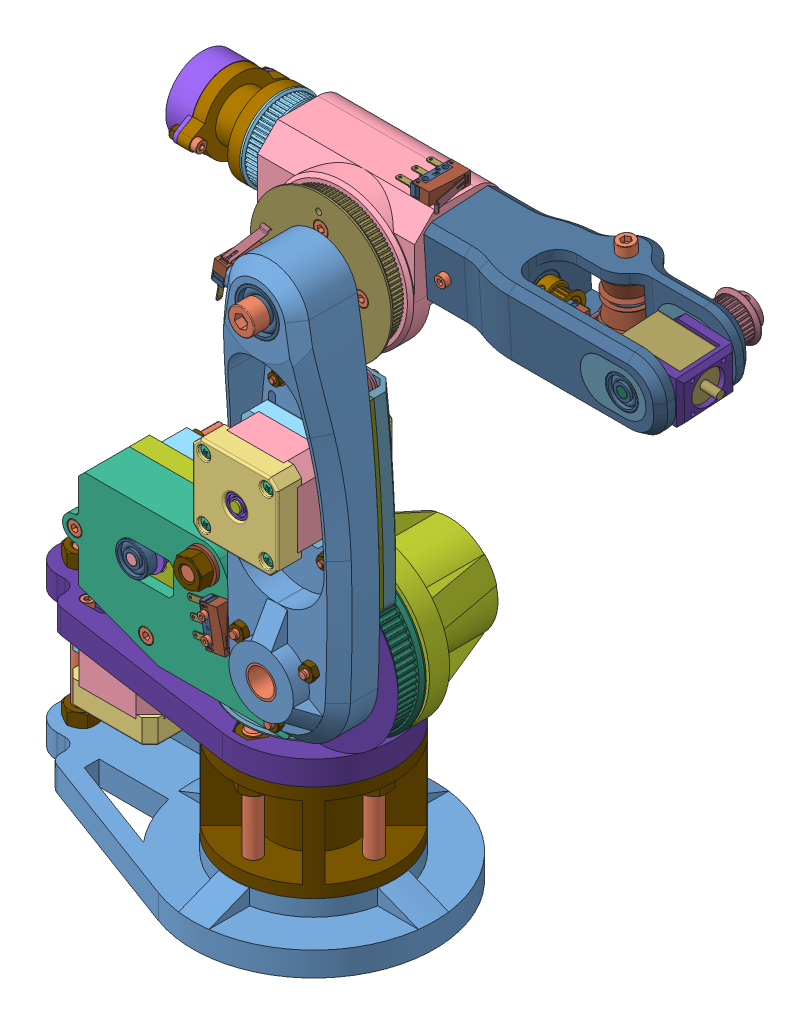
SolidWorks assembly Assem4_v2, configuration Default. Lengths in mm.
Overall size (329.84 338.53 142.9).
197 component instances, 53 part files, 399 mates.
Components (placement in the parent):
- Arm1v2-1: Arm1v2 [Default] at (144.3987 35.6213 88.0417) size (84.26 210 30)
- socket head cap screw_iso-2: socket head cap screw_iso [ISO 4762 M3 x 10 - 10N] at (128.8987 132.8213 85.0417) x (0 0 1) z (-1 0 0) size (13 5.5 5.5)
- socket head cap screw_iso-3: socket head cap screw_iso [ISO 4762 M3 x 10 - 10N] at (128.8987 101.8213 85.0417) x (0 0 1) z (-1 0 0) size (13 5.5 5.5)
- socket head cap screw_iso-4: socket head cap screw_iso [ISO 4762 M3 x 10 - 10N] at (159.8987 101.8213 85.0417) x (0 0 1) z (-1 0 0) size (13 5.5 5.5)
- socket head cap screw_iso-5: socket head cap screw_iso [ISO 4762 M3 x 10 - 10N] at (159.8987 132.8213 85.0417) x (0 0 1) z (-0.376004 -0.926618 0) size (13 5.5 5.5)
- NEMA 17 kiinalaiset-1: NEMA 17 kiinalaiset [Predeterminado] at (134.0032 112.7042 129.0417) x (-1 0 0) z (0 0 -1) size (42.3 42.3 56)
  - Base-1: Base [Predeterminado] at (-10.3955 4.6172 0) size (42.3 42.3 12)
  - Cuerpo-1: Cuerpo [Predeterminado] at (-10.3955 4.6172 10) size (42.3 42.3 16)
  - Tapa-1: Tapa [Predeterminado] at (-10.3955 4.6172 34) x (-1 0 0) z (0 0 -1) size (42.3 42.3 12)
  - pan cross head_am-1: pan cross head_am [B18.6.7M - M3 x 0.5 x 5 Type I Cross Recessed PHMS --5N] at (5.1045 20.1172 0.6) x (0 0 1) z (-0.896 0.444054 0) size (7.37 5.6 5.6)
  - pan cross head_am-2: pan cross head_am [B18.6.7M - M3 x 0.5 x 5 Type I Cross Recessed PHMS --5N] at (-25.8955 20.1172 0.6) x (0 0 1) z (-0.859432 0.51125 0) size (7.37 5.6 5.6)
  - pan cross head_am-3: pan cross head_am [B18.6.7M - M3 x 0.5 x 5 Type I Cross Recessed PHMS --5N] at (-25.8955 -10.8828 0.6) x (0 0 1) z (-0.91385 -0.406051 0) size (7.37 5.6 5.6)
  - pan cross head_am-4: pan cross head_am [B18.6.7M - M3 x 0.5 x 5 Type I Cross Recessed PHMS --5N] at (5.1045 -10.8828 0.6) x (0 0 1) z (-0.883632 0.468182 0) size (7.37 5.6 5.6)
  - Eje-1: Eje [Predeterminado] at (-10.3955 4.6172 0) x (0.574856 0.818255 0) z (0 0 1) size (5 5 56)
  - instrument ball bearing_68_am-2: instrument ball bearing_68_am [AFBMA 12.1.4.1 - 0050-11 - 10,SI,NC,10_68] at (-10.3955 4.6172 34) x (0 0 -1) z (0.925764 0.378103 0) size (3 11 11)
  - instrument ball bearing_68_am-4: instrument ball bearing_68_am [AFBMA 12.1.4.1 - 0050-11 - 10,SI,NC,10_68] at (-10.3955 4.6172 2.401) x (0 0 1) z (-0.993665 0.112385 0) size (3 11 11)
- GT2_16T_13x14-1: GT2_16T_13x14 [Конфигурация1] at (144.3987 117.3213 90.7117) x (0 0 -1) z (0.99998 0.006396 0) size (14.1 13 13)
- angular contact ball bearing_68_iso-1: angular contact ball bearing_68_iso [ISO 15 ABB - 108 - 8,SI,NC,8_68] at (144.3987 195.6213 91.5417) x (0 0 1) z (-0.999999 0.001328 0) size (7 22 22)
- angular contact ball bearing_68_iso-2: angular contact ball bearing_68_iso [ISO 15 ABB - 108 - 8,SI,NC,8_68] at (144.3987 195.6213 114.5417) x (0 0 -1) z (0.614558 -0.788871 0) size (7 22 22)
- socket head cap screw_iso-7: socket head cap screw_iso [ISO 4762 M8 x 80 - 28N] at (144.3987 195.6213 126.0417) x (0 0 -1) z (-0.988385 0.151973 0) size (88 13 13)
- plain washer normal grade a_iso-2: plain washer normal grade a_iso [Washer ISO 7089 - 8] at (144.3987 195.6213 88.0417) x (0 0 1) z (-0.999209 -0.03976 0) size (1.6 16 16)
- Pulley100Tv5-1: Pulley100Tv5 [Default] at (144.3987 195.6213 76.8417) x (0 0 1) z (0 1 0) size (15.6 70 70)
- socket head cap screw_iso-9: socket head cap screw_iso [ISO 4762 M3 x 25 - 18N] at (156.3987 150.6213 71.0417) x (0 0 1) z (-0.617239 0.786775 0) size (28 5.5 5.5)
- socket head cap screw_iso-10: socket head cap screw_iso [ISO 4762 M3 x 25 - 18N] at (132.3987 150.6213 71.0417) x (0 0 1) z (0.109591 0.993977 0) size (28 5.5 5.5)
- plain washer normal grade a_iso-4: plain washer normal grade a_iso [Washer ISO 7089 - 3] at (132.3987 150.6213 86.0417) x (0 0 1) z (-1 0 0) size (0.5 7 7)
- plain washer normal grade a_iso-5: plain washer normal grade a_iso [Washer ISO 7089 - 3] at (132.3987 150.6213 76.5417) x (0 0 1) z (-1 0 0) size (0.5 7 7)
- plain washer normal grade a_iso-6: plain washer normal grade a_iso [Washer ISO 7089 - 3] at (156.3987 150.6213 86.0417) x (0 0 1) z (-1 0 0) size (0.5 7 7)
- plain washer normal grade a_iso-7: plain washer normal grade a_iso [Washer ISO 7089 - 3] at (156.3987 150.6213 76.5417) x (0 0 1) z (-1 0 0) size (0.5 7 7)
- Toothless pulley 16t gt2-1: Toothless pulley 16t gt2 [Default] at (132.3987 150.6213 76.5417) x (0.593276 -0.804999 0) z (0 0 1) size (13 13 9)
- Toothless pulley 16t gt2-2: Toothless pulley 16t gt2 [Default] at (156.3987 150.6213 76.5417) x (0.93408 -0.357064 0) z (0 0 1) size (13 13 9)
- Arm 2.3-1: Arm 2.3 [Default] at (144.3987 35.6213 74.0417) x (0 0 1) z (-1 0 0) size (12 90.22 61.67)
- HTD3M 80T-1: HTD3M 80T [Default] at (144.3987 35.6213 86.4417) x (-0.5 -0.866025 0) z (0 0 -1) size (80 80 12.4)
- Arm 4.3-1: Arm 4.3 [Default] at (144.3987 35.6213 88.0417) x (0 0 -1) z (1 0 0) size (12 90.22 61.67)
- HTD80T 2mm spacer-1: HTD80T 2mm spacer [Default] at (144.3987 35.6213 88.0417) x (0.5 -0.866025 0) z (0.866025 0.5 0) size (80 1.6 80)
- socket head cap screw_iso-11: socket head cap screw_iso [ISO 4762 M3 x 25 - 18N] at (156.3987 83.6213 71.0417) x (0 0 1) z (-0.617239 0.786775 0) size (28 5.5 5.5)
- socket head cap screw_iso-12: socket head cap screw_iso [ISO 4762 M3 x 25 - 18N] at (132.3987 83.6213 71.0417) x (0 0 1) z (-0.617239 0.786775 0) size (28 5.5 5.5)
- socket head cap screw_iso-14: socket head cap screw_iso [ISO 4762 M4 x 35 - 20N] at (161.7192 45.6213 74.0417) x (0 0 1) z (-1 0 0) size (39 7 7)
- socket head cap screw_iso-15: socket head cap screw_iso [ISO 4762 M4 x 35 - 20N] at (127.0782 45.6213 74.0417) x (0 0 1) z (-1 0 0) size (39 7 7)
- socket head cap screw_iso-16: socket head cap screw_iso [ISO 4762 M4 x 35 - 20N] at (144.3987 15.6213 74.0417) x (0 0 1) z (-1 0 0) size (39 7 7)
- hex nut style 1 gradeab_iso-2: hex nut style 1 gradeab_iso [ISO - 4032 - M4 - W - N] at (161.7192 45.6213 108.0417) x (-0.89075 -0.454494 0) z (0 0 -1) size (7 8.08 3.2)
- hex nut style 1 gradeab_iso-3: hex nut style 1 gradeab_iso [ISO - 4032 - M4 - W - N] at (144.3987 15.6213 108.0417) x (-0.861185 -0.508291 0) z (0 0 -1) size (7 8.08 3.2)
- hex nut style 1 gradeab_iso-4: hex nut style 1 gradeab_iso [ISO - 4032 - M4 - W - N] at (127.0782 45.6213 108.0417) x (-0.923728 -0.383049 0) z (0 0 -1) size (7 8.08 3.2)
- plain washer normal grade a_iso-12: plain washer normal grade a_iso [Washer ISO 7089 - 3] at (132.3987 150.6213 95.0417) x (0 0 -1) z (1 0 0) size (0.5 7 7)
- plain washer normal grade a_iso-13: plain washer normal grade a_iso [Washer ISO 7089 - 3] at (156.3987 150.6213 95.0417) x (0 0 -1) z (1 0 0) size (0.5 7 7)
- plain washer normal grade a_iso-14: plain washer normal grade a_iso [Washer ISO 7089 - 3] at (132.3987 83.6213 95.0417) x (0 0 -1) z (1 0 0) size (0.5 7 7)
- plain washer normal grade a_iso-15: plain washer normal grade a_iso [Washer ISO 7089 - 3] at (156.3987 83.6213 95.0417) x (0 0 -1) z (1 0 0) size (0.5 7 7)
- hex nut style 1 gradeab_iso-6: hex nut style 1 gradeab_iso [ISO - 4032 - M3 - W - N] at (156.3987 150.6213 95.5417) x (-0.938673 -0.34481 0) z (0 0 -1) size (5.5 6.35 2.4)
- hex nut style 1 gradeab_iso-7: hex nut style 1 gradeab_iso [ISO - 4032 - M3 - W - N] at (132.3987 150.6213 95.5417) x (-0.945652 -0.32518 0) z (0 0 -1) size (5.5 6.35 2.4)
- hex nut style 1 gradeab_iso-8: hex nut style 1 gradeab_iso [ISO - 4032 - M3 - W - N] at (132.3987 83.6213 95.5417) x (-0.632186 -0.774817 0) z (0 0 -1) size (5.5 6.35 2.4)
- hex nut style 1 gradeab_iso-11: hex nut style 1 gradeab_iso [ISO - 4032 - M3 - W - N] at (156.3987 83.6213 95.5417) x (-0.632186 -0.774817 0) z (0 0 -1) size (5.5 6.35 2.4)
- angular contact ball bearing_68_iso-3: angular contact ball bearing_68_iso [ISO 15 ABB - 1015 - 12,SI,NC,12_68] at (174.8987 210.6213 52.4417) x (1 0 0) z (0 -0.976606 0.215038) size (9 32 32)
- angular contact ball bearing_68_iso-4: angular contact ball bearing_68_iso [ISO 15 ABB - 1015 - 12,SI,NC,12_68] at (105.8987 210.6213 52.4417) x (1 0 0) z (0 -0.4108 -0.911725) size (9 32 32)
- 100mm aluputki-1: 100mm aluputki [Default] at (66.1987 210.6213 52.4417) x (1 0 0) z (0 0.412587 -0.910918) size (145 15 15)
- 90mm aluputki-1: 90mm aluputki [Default] at (144.3987 35.6213 26.0417) x (-0.632641 -0.774445 0) z (0 0 1) size (15 15 90)
- angular contact ball bearing_68_iso-5: angular contact ball bearing_68_iso [ISO 15 ABB - 1015 - 12,SI,NC,12_68] at (144.3987 35.6213 67.9417) x (0 0 1) z (-0.817534 0.575881 0) size (9 32 32)
- angular contact ball bearing_68_iso-6: angular contact ball bearing_68_iso [ISO 15 ABB - 1015 - 12,SI,NC,12_68] at (144.3987 35.6213 26.9417) x (0 0 1) z (-0.997702 0.067753 0) size (9 32 32)
- 15mm 1.6 rikka-1: 15mm 1.6 rikka [Default] at (144.3987 35.6213 74.0417) x (0 0 -1) z (1 -0.000633 0) size (1.6 22 22)
- socket head cap screw_iso-23: socket head cap screw_iso [ISO 4762 M8 x 40 - 28N] at (94.3987 50.6213 54.4417) x (0 0 1) z (-0.999928 0.012039 0) size (48 13 13)
- angular contact ball bearing_68_iso-7: angular contact ball bearing_68_iso [ISO 15 ABB - 108 - 8,SI,NC,8_68] at (94.3987 50.6213 77.5417) x (0 0 -1) z (0.936997 0.349338 0) size (7 22 22)
- Arm2Mountv2-1: Arm2Mountv2 [Default] at (144.3987 195.6213 76.8417) x (0 0 -1) z (1 0 0) size (46 80 78)
- Pulley60Tv2-1: Pulley60Tv2 [Default] at (100.1987 210.6213 52.4417) x (0 0.659878 0.751372) z (-1 0 0) size (40 40 10)
- GT2_16T_13x14-2: GT2_16T_13x14 [Конфигурация1] at (104.8687 168.7922 48.8417) x (-1 0 0) z (0 -0.490303 -0.871552) size (14.1 13 13)
- 15mm rikka 1.2mm-1: 15mm rikka 1.2mm [Default] at (101.3987 210.6213 52.4417) x (0 -0.416782 0.909006) z (-1 0 0) size (20 20 1.2)
- Nema 14 stepper-1: Nema 14 stepper [Default] at (129.3987 168.7922 48.8417) x (0 0 1) z (-1 0 0) size (35.2 35.2 32.5)
- Nema 14 Round stepper-2: Nema 14 Round stepper [Default] at (51.6987 210.6213 52.4417) x (0 0.064696 -0.997905) z (1 0 0) size (50.5 36.5 20)
- Motor 5 adapter-1: Motor 5 adapter [Default] at (90.1987 210.6213 52.4417) x (-1 0 0) z (0 0.064696 -0.997905) size (26 40 50.5)
- socket head cap screw_iso-33: socket head cap screw_iso [ISO 4762 M3 x 12 - 12N] at (73.1987 209.2012 74.3457) x (-1 0 0) z (0 -0.223084 0.974799) size (15 5.5 5.5)
- socket head cap screw_iso-34: socket head cap screw_iso [ISO 4762 M3 x 12 - 12N] at (73.1987 212.0414 30.5377) x (-1 0 0) z (0 -0.996697 0.081212) size (15 5.5 5.5)
- hex nut style 1 gradeab_iso-15: hex nut style 1 gradeab_iso [ISO - 4032 - M3 - W - N] at (62.1987 212.0414 30.5377) x (0 -0.893584 -0.448895) z (1 0 0) size (5.5 6.35 2.4)
- hex nut style 1 gradeab_iso-16: hex nut style 1 gradeab_iso [ISO - 4032 - M3 - W - N] at (62.1987 209.2012 74.3457) x (0 -0.971525 -0.236939) z (1 0 0) size (5.5 6.35 2.4)
- plain washer normal grade a_iso-17: plain washer normal grade a_iso [Washer ISO 7089 - 8] at (94.3987 50.6213 72.4417) x (0 0 -1) z (1 0 0) size (1.6 16 16)
- plain washer normal grade a_iso-18: plain washer normal grade a_iso [Washer ISO 7089 - 8] at (94.3987 50.6213 89.6417) x (0 0 1) z (-1 0 0) size (1.6 16 16)
- angular contact ball bearing_68_iso-8: angular contact ball bearing_68_iso [ISO 15 ABB - 108 - 8,SI,NC,8_68] at (94.3987 50.6213 84.5417) x (0 0 -1) z (0.994052 0.108909 0) size (7 22 22)
- plain washer normal grade a_iso-20: plain washer normal grade a_iso [Washer ISO 7089 - 8] at (94.3987 50.6213 94.6417) x (0 0 -1) z (0.534163 0.845382 0) size (1.6 16 16)
- hex nut style 1 gradeab_iso-18: hex nut style 1 gradeab_iso [ISO - 4032 - M8 - W - N] at (94.3987 50.6213 96.2417) x (-0.975025 0.222094 0) z (0 0 -1) size (13 15.01 6.8)
- Microswitch-SS-3GL13SL-1: Microswitch-SS-3GL13SL [Default] at (90.1948 35.3075 79.4243) x (0.173648 -0.984808 0) z (0 0 1) size (23.17 24.53 6.3)
  - limit-switch-bottomcase-1: limit-switch-bottomcase [Default] at (4.8379 12.1903 15.2174) size (19.75 5.4 6.2)
  - limit-switch-top-case-1: limit-switch-top-case [Default] at (4.8379 12.1903 15.2174) size (19.75 9.81 6.3)
  - pins-1: pins [Default] at (4.7048 12.1903 18.0824) size (18.65 8.8 0.47)
  - switch_lever-1: switch_lever [Default] at (4.2786 20.8228 20.3174) x (0 0 -1) z (0.981158 -0.193205 0) size (4 3.58 20.93)
- socket head cap screw_iso-36: socket head cap screw_iso [ISO 4762 M2 x 10 - 10N] at (101.319 35.6213 102.8417) x (0 0 -1) z (1 0 0) size (12 3.8 3.8)
- socket head cap screw_iso-37: socket head cap screw_iso [ISO 4762 M2 x 10 - 10N] at (103.0555 25.7732 102.8417) x (0 0 -1) z (1 0 0) size (12 3.8 3.8)
- socket head cap screw_iso-39: socket head cap screw_iso [ISO 4762 M3 x 8 - 8N] at (101.3987 181.7922 35.8417) x (1 0 0) z (0 -0.369885 0.929078) size (11 5.5 5.5)
- socket head cap screw_iso-40: socket head cap screw_iso [ISO 4762 M3 x 8 - 8N] at (101.3987 181.7922 61.8417) x (1 0 0) z (0 -0.369885 0.929078) size (11 5.5 5.5)
- socket head cap screw_iso-41: socket head cap screw_iso [ISO 4762 M3 x 8 - 8N] at (101.3987 155.7922 61.8417) x (1 0 0) z (0 -0.369885 0.929078) size (11 5.5 5.5)
- socket head cap screw_iso-42: socket head cap screw_iso [ISO 4762 M3 x 8 - 8N] at (101.3987 155.7922 35.8417) x (1 0 0) z (0 0.072717 0.997353) size (11 5.5 5.5)
- socket head cap screw_iso-44: socket head cap screw_iso [ISO 4762 M4 x 16 - 16N] at (144.3987 215.6213 86.4417) x (0 0 -1) z (1 0 0) size (20 7 7)
- socket head cap screw_iso-46: socket head cap screw_iso [ISO 4762 M4 x 16 - 16N] at (164.3987 195.6213 86.4417) x (0 0 -1) z (1 0 0) size (20 7 7)
- socket head cap screw_iso-47: socket head cap screw_iso [ISO 4762 M4 x 16 - 16N] at (144.3987 175.6213 86.4417) x (0 0 -1) z (1 0 0) size (20 7 7)
- socket head cap screw_iso-48: socket head cap screw_iso [ISO 4762 M4 x 16 - 16N] at (124.3987 195.6213 86.4417) x (0 0 -1) z (0.806628 0.591059 0) size (20 7 7)
- hex nut style 1 gradeab_iso-19: hex nut style 1 gradeab_iso [ISO - 4032 - M8 - W - N] at (144.3987 195.6213 45.8417) x (0.866025 -0.5 0) z (0 0 1) size (13 15.01 6.8)
- Microswitch-SS-3GL13SL-2: Microswitch-SS-3GL13SL [Default] at (133.5542 178.7224 93.9191) x (0 0 1) z (-0.985156 0.171661 0) size (23.17 24.53 6.3)
  - limit-switch-bottomcase-1: limit-switch-bottomcase [Default] at (4.8379 12.1903 15.2174) size (19.75 5.4 6.2)
  - limit-switch-top-case-1: limit-switch-top-case [Default] at (4.8379 12.1903 15.2174) size (19.75 9.81 6.3)
  - pins-1: pins [Default] at (4.7048 12.1903 18.0824) size (18.65 8.8 0.47)
  - switch_lever-1: switch_lever [Default] at (4.2786 20.8228 20.3174) x (0 0 -1) z (0.981158 -0.193205 0) size (4 3.58 20.93)
- Pulley100TBase-2: Pulley100TBase [Default] at (106.8987 -6.3787 52.4417) x (0 -1 0) z (1 0 0) size (9.3 70 70)
- socket head cap screw_iso-50: socket head cap screw_iso [ISO 4762 M4 x 35 - 20N] at (65.8987 5.6213 94.6417) x (0 0 -1) z (0.847074 -0.531475 0) size (39 7 7)
- hex nut style 1 gradeab_iso-21: hex nut style 1 gradeab_iso [ISO - 4032 - M4 - W - N] at (65.8987 5.6213 62.4417) x (-0.520571 -0.853818 0) z (0 0 1) size (7 8.08 3.2)
- socket head cap screw_iso-54: socket head cap screw_iso [ISO 4762 M4 x 30 - 20N] at (30.3987 34.1213 94.6417) x (0 0 -1) z (0.979653 0.200699 0) size (34 7 7)
- hex nut style 1 gradeab_iso-22: hex nut style 1 gradeab_iso [ISO - 4032 - M4 - W - N] at (30.3987 34.1213 67.4417) x (0.5 -0.866025 0) z (0 0 1) size (7 8.08 3.2)
- hex nut style 1 gradeab_iso-23: hex nut style 1 gradeab_iso [ISO - 4032 - M8 - W - N] at (106.8987 42.6213 52.4417) x (0.866025 0 -0.5) z (0 -1 0) size (13 15.01 6.8)
- thrust ball bearing_68_iso-1: thrust ball bearing_68_iso [ISO 104 - 112035 - B,14,SI,NC,14_68] at (106.8987 -17.6787 52.4417) x (0 -1 0) z (-0.999778 0 -0.021086) size (10 35 35)
- thrust ball bearing_68_iso-2: thrust ball bearing_68_iso [ISO 104 - 112035 - B,14,SI,NC,14_68] at (106.8987 -81.6787 52.4417) x (0 1 0) z (0.068397 0 0.997658) size (10 35 35)
- Bottom spacer-1: Bottom spacer [Default] at (106.8987 -4.3787 52.4417) x (0.893445 0 -0.449173) z (-0.449173 0 -0.893445) size (70 2 70)
- Baseplate-1: Baseplate [Default] at (106.8987 -31.6787 52.4417) x (-1 0 0) z (0 0 -1) size (167.5 12 80)
- Bottom Tube-1: Bottom Tube [Default] at (106.8987 -31.6787 52.4417) x (0 0 -1) z (-1 0 0) size (80 48 80)
- angular contact ball bearing_68_iso-9: angular contact ball bearing_68_iso [ISO 15 ABB - 1015 - 12,SI,NC,12_68] at (106.8987 -27.1787 52.4417) x (0 -1 0) z (0 0 1) size (9 32 32)
- angular contact ball bearing_68_iso-10: angular contact ball bearing_68_iso [ISO 15 ABB - 1015 - 12,SI,NC,12_68] at (106.8987 -72.1787 52.4417) x (0 -1 0) z (0.009581 0 0.999954) size (9 32 32)
- Bottom support-1: Bottom support [Default] at (106.8987 -87.6787 52.4417) x (-1 0 0) z (0 0 -1) size (187.5 20 120)
- socket head cap screw_iso-58: socket head cap screw_iso [ISO 4762 M4 x 20 - 20N] at (131.8987 -15.6787 52.4417) x (0 1 0) z (0 0 1) size (24 7 7)
- hex nut style 1 gradeab_iso-24: hex nut style 1 gradeab_iso [ISO - 4032 - M4 - W - N] at (131.8987 5.6213 52.4417) x (-0.994978 0 0.100092) z (0 -1 0) size (7 8.08 3.2)
- NEMA 17 kiinalaiset-2: NEMA 17 kiinalaiset [Predeterminado] at (15.2032 -63.6787 47.8246) x (-1 0 0) z (0 1 0) size (42.3 42.3 56)
  - Base-1: Base [Predeterminado] at (-10.3955 4.6172 0) size (42.3 42.3 12)
  - Cuerpo-1: Cuerpo [Predeterminado] at (-10.3955 4.6172 10) size (42.3 42.3 16)
  - Tapa-1: Tapa [Predeterminado] at (-10.3955 4.6172 34) x (-1 0 0) z (0 0 -1) size (42.3 42.3 12)
  - pan cross head_am-1: pan cross head_am [B18.6.7M - M3 x 0.5 x 5 Type I Cross Recessed PHMS --5N] at (5.1045 20.1172 0.6) x (0 0 1) z (-0.896 0.444054 0) size (7.37 5.6 5.6)
  - pan cross head_am-2: pan cross head_am [B18.6.7M - M3 x 0.5 x 5 Type I Cross Recessed PHMS --5N] at (-25.8955 20.1172 0.6) x (0 0 1) z (-0.859432 0.51125 0) size (7.37 5.6 5.6)
  - pan cross head_am-3: pan cross head_am [B18.6.7M - M3 x 0.5 x 5 Type I Cross Recessed PHMS --5N] at (-25.8955 -10.8828 0.6) x (0 0 1) z (-0.91385 -0.406051 0) size (7.37 5.6 5.6)
  - pan cross head_am-4: pan cross head_am [B18.6.7M - M3 x 0.5 x 5 Type I Cross Recessed PHMS --5N] at (5.1045 -10.8828 0.6) x (0 0 1) z (-0.883632 0.468182 0) size (7.37 5.6 5.6)
  - Eje-1: Eje [Predeterminado] at (-10.3955 4.6172 0) x (0.574856 0.818255 0) z (0 0 1) size (5 5 56)
  - instrument ball bearing_68_am-2: instrument ball bearing_68_am [AFBMA 12.1.4.1 - 0050-11 - 10,SI,NC,10_68] at (-10.3955 4.6172 34) x (0 0 -1) z (0.925764 0.378103 0) size (3 11 11)
  - instrument ball bearing_68_am-4: instrument ball bearing_68_am [AFBMA 12.1.4.1 - 0050-11 - 10,SI,NC,10_68] at (-10.3955 4.6172 2.401) x (0 0 1) z (-0.993665 0.112385 0) size (3 11 11)
- socket head cap screw_iso-60: socket head cap screw_iso [ISO 4762 M3 x 10 - 10N] at (10.0987 -19.6787 36.9417) x (0 -1 0) z (0.275126 0 0.961408) size (13 5.5 5.5)
- socket head cap screw_iso-61: socket head cap screw_iso [ISO 4762 M3 x 10 - 10N] at (10.0987 -19.6787 67.9417) x (0 -1 0) z (0 0 1) size (13 5.5 5.5)
- socket head cap screw_iso-62: socket head cap screw_iso [ISO 4762 M3 x 10 - 10N] at (41.0987 -19.6787 36.9417) x (0 -1 0) z (0 0 1) size (13 5.5 5.5)
- socket head cap screw_iso-63: socket head cap screw_iso [ISO 4762 M3 x 10 - 10N] at (41.0987 -19.6787 67.9417) x (0 -1 0) z (0 0 1) size (13 5.5 5.5)
- GT2_16T_13x14-3: GT2_16T_13x14 [Конфигурация1] at (25.5987 -20.2487 52.4417) x (0 1 0) z (0 0 1) size (14.1 13 13)
- socket head cap screw_iso-65: socket head cap screw_iso [ISO 4762 M8 x 70 - 28N] at (106.8987 -97.6787 22.4417) x (0 1 0) z (0 0 1) size (78 13 13)
- socket head cap screw_iso-66: socket head cap screw_iso [ISO 4762 M8 x 70 - 28N] at (76.8987 -97.6787 52.4417) x (0 1 0) z (0 0 1) size (78 13 13)
- socket head cap screw_iso-67: socket head cap screw_iso [ISO 4762 M8 x 70 - 28N] at (106.8987 -97.6787 82.4417) x (0 1 0) z (0 0 1) size (78 13 13)
- socket head cap screw_iso-68: socket head cap screw_iso [ISO 4762 M8 x 70 - 28N] at (136.8987 -97.6787 52.4417) x (0 1 0) z (0 0 1) size (78 13 13)
- hex nut style 1 gradeab_iso-26: hex nut style 1 gradeab_iso [ISO - 4032 - M8 - D - N] at (106.8987 -44.4787 22.4417) x (1 0 0) z (0 -1 0) size (13 15.01 6.8)
- hex nut style 1 gradeab_iso-27: hex nut style 1 gradeab_iso [ISO - 4032 - M8 - D - N] at (136.8987 -44.4787 52.4417) x (1 0 0) z (0 -1 0) size (13 15.01 6.8)
- hex nut style 1 gradeab_iso-28: hex nut style 1 gradeab_iso [ISO - 4032 - M8 - D - N] at (106.8987 -44.4787 82.4417) x (1 0 0) z (0 -1 0) size (13 15.01 6.8)
- hex nut style 1 gradeab_iso-29: hex nut style 1 gradeab_iso [ISO - 4032 - M8 - D - N] at (76.8987 -43.4787 52.4417) x (1 0 0) z (0 -1 0) size (13 15.01 6.8)
- hex nut style 1 gradeab_iso-30: hex nut style 1 gradeab_iso [ISO - 4032 - M8 - D - N] at (106.8987 -20.8787 82.4417) x (0.866025 0 -0.5) z (0 1 0) size (13 15.01 6.8)
- hex nut style 1 gradeab_iso-31: hex nut style 1 gradeab_iso [ISO - 4032 - M8 - D - N] at (136.8987 -27.6787 52.4417) x (1 0 0) z (0 -1 0) size (13 15.01 6.8)
- hex nut style 1 gradeab_iso-32: hex nut style 1 gradeab_iso [ISO - 4032 - M8 - D - N] at (106.8987 -20.8787 22.4417) x (-0.866025 0 0.5) z (0 1 0) size (13 15.01 6.8)
- hex nut style 1 gradeab_iso-33: hex nut style 1 gradeab_iso [ISO - 4032 - M8 - D - N] at (76.8987 -27.6787 52.4417) x (1 0 0) z (0 -1 0) size (13 15.01 6.8)
- hex bolt gradeab_iso-2: hex bolt gradeab_iso [ISO 4014 - M8 x 80 x 80-N] at (-8.1013 -98.9787 52.4417) x (0 1 0) z (0 0 1) size (85.3 15.01 13)
- hex nut style 1 gradeab_iso-35: hex nut style 1 gradeab_iso [ISO - 4032 - M8 - D - N] at (-8.1013 -87.6787 52.4417) x (1 0 0) z (0 -1 0) size (13 15.01 6.8)
- hex nut style 1 gradeab_iso-36: hex nut style 1 gradeab_iso [ISO - 4032 - M8 - D - N] at (-8.1013 -38.4787 52.4417) x (1 0 0) z (0 -1 0) size (13 15.01 6.8)
- hex nut style 1 gradeab_iso-37: hex nut style 1 gradeab_iso [ISO - 4032 - M8 - D - N] at (-8.1013 -19.6787 52.4417) x (1 0 0) z (0 -1 0) size (13 15.01 6.8)
- Nema 17 planetary 5 to 1 gearbox-1: Nema 17 planetary 5 to 1 gearbox [Default] at (59.3987 35.6213 -13.8583) size (42.3 42.3 79.3)
- HTD pulley adapter-1: HTD pulley adapter [Default] at (59.3987 35.6213 54.4417) x (0.999676 0.02547 0) z (0 0 1) size (12 12 41)
- Motor1 spacer-1: Motor1 spacer [Default] at (59.3987 35.6213 47.4417) size (45 45 15)
- socket head cap screw_iso-70: socket head cap screw_iso [ISO 4762 M3 x 10 - 10N] at (49.4992 45.5208 57.4417) x (0 0 -1) z (1 0 0) size (13 5.5 5.5)
- socket head cap screw_iso-71: socket head cap screw_iso [ISO 4762 M3 x 10 - 10N] at (69.2982 45.5208 57.4417) x (0 0 -1) z (1 0 0) size (13 5.5 5.5)
- socket head cap screw_iso-72: socket head cap screw_iso [ISO 4762 M3 x 10 - 10N] at (69.2982 25.7218 57.4417) x (0 0 -1) z (1 0 0) size (13 5.5 5.5)
- socket head cap screw_iso-73: socket head cap screw_iso [ISO 4762 M3 x 10 - 10N] at (49.4992 25.7218 57.4417) x (0 0 -1) z (1 0 0) size (13 5.5 5.5)
- socket head cap screw_iso-75: socket head cap screw_iso [ISO 4762 M4 x 35 - 20N] at (41.8987 53.1213 72.4417) x (0 0 -1) z (1 0 0) size (39 7 7)
- socket head cap screw_iso-76: socket head cap screw_iso [ISO 4762 M4 x 35 - 20N] at (76.8987 53.1213 72.4417) x (0 0 -1) z (1 0 0) size (39 7 7)
- socket head cap screw_iso-77: socket head cap screw_iso [ISO 4762 M4 x 35 - 20N] at (41.8987 18.1213 72.4417) x (0 0 -1) z (1 0 0) size (39 7 7)
- socket head cap screw_iso-78: socket head cap screw_iso [ISO 4762 M4 x 35 - 20N] at (76.8987 18.1213 72.4417) x (0 0 -1) z (1 0 0) size (39 7 7)
- hex nut style 1 gradeab_iso-39: hex nut style 1 gradeab_iso [ISO - 4032 - M4 - D - N] at (76.8987 53.1213 44.2417) x (0.923728 0.383049 0) z (0 0 -1) size (7 8.08 3.2)
- hex nut style 1 gradeab_iso-40: hex nut style 1 gradeab_iso [ISO - 4032 - M4 - D - N] at (41.8987 53.1213 44.2417) x (0.923728 0.383049 0) z (0 0 -1) size (7 8.08 3.2)
- hex nut style 1 gradeab_iso-41: hex nut style 1 gradeab_iso [ISO - 4032 - M4 - D - N] at (41.8987 18.1213 44.2417) x (0.923728 0.383049 0) z (0 0 -1) size (7 8.08 3.2)
- hex nut style 1 gradeab_iso-42: hex nut style 1 gradeab_iso [ISO - 4032 - M4 - D - N] at (76.8987 18.1213 44.2417) x (0.923728 0.383049 0) z (0 0 -1) size (7 8.08 3.2)
- Basewall cover v2-1: Basewall cover v2 [Default] at (144.3987 35.6213 72.4417) size (112.64 65 22.2)
- BaseWall_2_v2-1: BaseWall_2_v2 [Default] at (144.3987 35.6213 62.4417) x (0 0 1) z (-1 0 0) size (55 80 160)
- 3M HTD 16T 6mm Bore-1: 3M HTD 16T 6mm Bore [Default] at (59.3987 35.6213 70.2417) x (-0.898484 0.439007 0) z (0 0 1) size (18 18 18)
- angular contact ball bearing_68_iso-11: angular contact ball bearing_68_iso [ISO 15 ABB - 025 - 8,SI,NC,8_68] at (59.3987 35.6213 92.9417) x (0 0 -1) z (-0.141497 0.989939 0) size (5 16 16)
- 6mm akseli-1: 6mm akseli [Default] at (71.6987 210.6213 52.4417) x (0 -0.346295 -0.938126) z (1 0 0) size (5 5 170)
- angular contact ball bearing_68_iso-12: angular contact ball bearing_68_iso [ISO 15 ABB - 025 - 8,SI,NC,8_68] at (218.8987 210.6213 52.4417) x (1 0 0) z (0 0.914388 0.40484) size (5 16 16)
- GT2_16T_13x14-4: GT2_16T_13x14 [Конфигурация1] at (221.3987 210.6213 52.4417) x (1 0 0) z (0 -0.758002 0.652253) size (14.1 13 13)
- Microswitch-SS-3GL13SL-4: Microswitch-SS-3GL13SL [Default] at (158.789 252.0387 61.5893) x (0 0 -1) z (0 -1 0) size (23.17 24.53 6.3)
  - limit-switch-bottomcase-1: limit-switch-bottomcase [Default] at (4.8379 12.1903 15.2174) size (19.75 5.4 6.2)
  - limit-switch-top-case-1: limit-switch-top-case [Default] at (4.8379 12.1903 15.2174) size (19.75 9.81 6.3)
  - pins-1: pins [Default] at (4.7048 12.1903 18.0824) size (18.65 8.8 0.47)
  - switch_lever-1: switch_lever [Default] at (4.2786 20.8228 20.3174) x (0 0 -1) z (0.981158 -0.193205 0) size (4 3.58 20.93)
- socket head cap screw_iso-84: socket head cap screw_iso [ISO 4762 M3 x 16 - 16N] at (190.3987 209.2627 73.3977) x (0 0.064696 -0.997905) z (-0.161809 -0.984755 -0.063843) size (19 5.5 5.5)
- socket head cap screw_iso-86: socket head cap screw_iso [ISO 4762 M3 x 12 - 12N] at (183.3987 191.1424 31.5173) x (0 0.758027 0.652223) z (0.967093 -0.16594 0.192859) size (15 5.5 5.5)
- Rotation arm V3-1: Rotation arm V3 [Default] at (180.3987 210.6213 52.4417) x (0 -0.064696 0.997905) z (1 0 0) size (56 35 122)
- socket head cap screw_iso-88: socket head cap screw_iso [ISO 4762 M5 x 40 - 22N] at (243.3987 234.3681 33.9393) x (0 -0.997905 -0.064696) z (0.99979 -0.001327 0.020473) size (45 8.5 8.5)
- angular contact ball bearing_68_iso-18: angular contact ball bearing_68_iso [ISO 15 ABB - 025 - 8,SI,NC,8_68] at (243.3987 220.8964 33.0659) x (0 0.997905 0.064696) z (0.241088 -0.062788 0.96847) size (5 16 16)
- angular contact ball bearing_68_iso-19: angular contact ball bearing_68_iso [ISO 15 ABB - 025 - 8,SI,NC,8_68] at (243.3987 215.9069 32.7424) x (0 0.997905 0.064696) z (0.251816 -0.062611 0.965748) size (5 16 16)
- angular contact ball bearing_68_iso-20: angular contact ball bearing_68_iso [ISO 15 ABB - 025 - 8,SI,NC,8_68] at (243.3987 207.9236 32.2248) x (0 0.997905 0.064696) z (0.268051 -0.062328 0.961386) size (5 16 16)
- angular contact ball bearing_68_iso-21: angular contact ball bearing_68_iso [ISO 15 ABB - 025 - 8,SI,NC,8_68] at (243.3987 202.9341 31.9013) x (0 0.997905 0.064696) z (0.243771 -0.062744 0.967801) size (5 16 16)
- plain washer normal grade a_iso-24: plain washer normal grade a_iso [Washer ISO 7089 - 5] at (243.3987 199.4414 31.6749) x (0 -0.997905 -0.064696) z (0.009718 -0.064693 0.997858) size (1 10 10)
- plain washer normal grade a_iso-25: plain washer normal grade a_iso [Washer ISO 7089 - 5] at (243.3987 223.3911 33.2276) x (0 -0.997905 -0.064696) z (0.009718 -0.064693 0.997858) size (1 10 10)
- GT2 hihna chamfer rulla-1: GT2 hihna chamfer rulla [Default] at (243.3987 214.909 32.6777) x (0.991292 0.008519 -0.131404) z (0.13168 -0.064133 0.989216) size (23 10 23)
- GT2 hihna chamfer rulla-2: GT2 hihna chamfer rulla [Default] at (243.3987 208.9215 32.2895) x (0.541355 -0.054396 0.839033) z (0.840794 0.035023 -0.540221) size (23 10 23)
- Nema8 Stepperi (banggood.com)-1: Nema8 Stepperi (banggood.com) [Default] at (268.814 211.274 52.484) x (0.046717 0.996815 0.064625) z (0.998908 -0.046619 -0.003022) size (20 20 40)
- Pulley32TGT2-1: Pulley32TGT2 [Default] at (282.7987 212.2387 27.4941) x (-0.976366 0.215672 0.013982) z (0 0.064696 -0.997905) size (23 23 15)
- Microswitch-SS-3GL13SL-5: Microswitch-SS-3GL13SL [Default] at (235.789 221.2627 46.7008) x (0 -0.997905 -0.064696) z (0 -0.064696 0.997905) size (23.17 24.53 6.3)
  - limit-switch-bottomcase-1: limit-switch-bottomcase [Default] at (4.8379 12.1903 15.2174) size (19.75 5.4 6.2)
  - limit-switch-top-case-1: limit-switch-top-case [Default] at (4.8379 12.1903 15.2174) size (19.75 9.81 6.3)
  - pins-1: pins [Default] at (4.7048 12.1903 18.0824) size (18.65 8.8 0.47)
  - switch_lever-1: switch_lever [Default] at (4.2786 20.8228 20.3174) x (0 0 -1) z (0.981158 -0.193205 0) size (4 3.58 20.93)
- bearing adapter J6 housing-1: bearing adapter J6 housing [Default] at (283.6987 209.1333 75.3935) x (-1 0 0) z (0 -0.997905 -0.064696) size (32.5 8 22.2)
- angular contact ball bearing_68_iso-22: angular contact ball bearing_68_iso [ISO 15 ABB - 025 - 8,SI,NC,8_68] at (282.7987 211.9476 31.9847) x (0 -0.064696 0.997905) z (0.837901 -0.544679 -0.035313) size (5 16 16)
- angular contact ball bearing_68_iso-23: angular contact ball bearing_68_iso [ISO 15 ABB - 025 - 8,SI,NC,8_68] at (282.7987 209.2951 72.8988) x (0 0.064696 -0.997905) z (-0.927048 0.374156 0.024257) size (5 16 16)
- bearing adapter J6 housing-2: bearing adapter J6 housing [Default] at (283.6987 212.1093 29.4899) x (-1 0 0) z (0 0.997905 0.064696) size (32.5 8 22.2)
- 5mm akseli 2-1: 5mm akseli 2 [Default] at (282.7987 209.1333 75.3935) x (0.997104 -0.075891 -0.00492) z (0.076051 0.995015 0.064509) size (5 13 5)
- 5mm akseli 1-1: 5mm akseli 1 [Default] at (282.7987 213.2092 12.5255) x (-0.216125 -0.97432 -0.063167) z (-0.976366 0.215672 0.013982) size (5 30 5)
- J6 kotelo-2: J6 kotelo [Default] at (272.2958 199.4756 61.7401) x (0 -0.064696 0.997905) z (-0.998908 0.046619 0.003022) size (28 22 30)
Mates (geometry in assembly coordinates):
- Concentric1: concentric: cylinder of Arm1v2-1 through (128.8987 132.8213 76.0209) axis (0 0 1) radius 1.75; cylinder of socket head cap screw_iso-2 through (128.8987 132.8213 53.2917) axis (0 0 -1) radius 2.75
- Coincident1: coincident: plane of Arm1v2-1 through (503.9807 132.9651 88.0417) normal (0 0 -1); plane of socket head cap screw_iso-2 through (128.8987 135.5713 88.0417) normal (0 0 1)
- Concentric2: concentric: cylinder of Arm1v2-1 through (128.8987 101.8213 76.0209) axis (0 0 1) radius 1.75; cylinder of socket head cap screw_iso-3 through (128.8987 101.8213 53.2917) axis (0 0 -1) radius 2.75
- Coincident2: coincident: plane of Arm1v2-1 through (503.9807 132.9651 88.0417) normal (0 0 -1); plane of socket head cap screw_iso-3 through (128.8987 104.5713 88.0417) normal (0 0 1)
- Concentric4: concentric: cylinder of Arm1v2-1 through (159.8987 132.8213 76.0209) axis (0 0 1) radius 1.75; cylinder of socket head cap screw_iso-5 through (159.8987 132.8213 53.2917) axis (0 0 -1) radius 2.75
- Concentric5: concentric: cylinder of socket head cap screw_iso-5 through (159.8987 132.8213 53.2917) axis (0 0 -1) radius 1.5; cylinder of NEMA 17 kiinalaiset-1/Tapa-1 through (159.8987 132.8213 99.5417) axis (0 0 -1) radius 1.5
- Concentric6: concentric: cylinder of socket head cap screw_iso-3 through (128.8987 101.8213 53.2917) axis (0 0 -1) radius 1.5; cylinder of NEMA 17 kiinalaiset-1/Tapa-1 through (128.8987 101.8213 99.5417) axis (0 0 -1) radius 1.5
- Coincident5: coincident: plane of Arm1v2-1 through (503.9807 132.9651 95.0417) normal (0 0 1); plane of NEMA 17 kiinalaiset-1/Tapa-1 through (144.3987 117.3213 95.0417) normal (0 0 -1)
- Concentric7: concentric: cylinder of NEMA 17 kiinalaiset-1/Eje-1 through (144.3987 117.3213 73.0417) axis (0 0 1) radius 2.5; cylinder of GT2_16T_13x14-1 through (144.3987 117.3213 90.7117) axis (0 0 -1) radius 2.5
- Concentric8: concentric: cylinder of Arm1v2-1 through (144.3987 195.6213 95.0417) axis (0 0 -1) radius 11.1; cylinder of angular contact ball bearing_68_iso-1 through (144.3987 195.6213 70.9042) axis (0 0 1) radius 11
- Coincident6: coincident: plane of Arm1v2-1 through (144.3987 195.6213 95.0417) normal (0 0 -1); plane of angular contact ball bearing_68_iso-1 through (144.4129 206.3213 95.0417) normal (0 0 1)
- Concentric10: concentric: cylinder of angular contact ball bearing_68_iso-2 through (144.3987 195.6213 135.1792) axis (0 0 -1) radius 6.1; cylinder of socket head cap screw_iso-7 through (144.3987 195.6213 157.7917) axis (0 0 1) radius 6.5
- Coincident8: coincident: plane of angular contact ball bearing_68_iso-2 through (149.2108 199.3701 118.0417) normal (0 0 1); plane of socket head cap screw_iso-7 through (143.4109 189.1968 118.0417) normal (0 0 -1)
- Concentric11: concentric: cylinder of angular contact ball bearing_68_iso-1 through (144.3987 195.6213 70.9042) axis (0 0 1) radius 6.1; cylinder of plain washer normal grade a_iso-2 through (144.3987 195.6213 53.1167) axis (0 0 -1) radius 4.2
- Coincident9: coincident: plane of angular contact ball bearing_68_iso-1 through (144.4068 201.7213 88.0417) normal (0 0 -1); plane of plain washer normal grade a_iso-2 through (144.2317 199.818 88.0417) normal (0 0 1)
- Concentric12: concentric: cylinder of socket head cap screw_iso-7 through (144.3987 195.6213 157.7917) axis (0 0 1) radius 4; cylinder of Pulley100Tv5-1 through (144.3987 195.6213 84.5417) axis (0 0 -1) radius 4
- Coincident10: coincident: plane of plain washer normal grade a_iso-2 through (144.0806 203.615 86.4417) normal (0 0 -1); plane of Pulley100Tv5-1 through (144.3987 195.6213 86.4417) normal (0 0 1)
- Concentric13: concentric: cylinder of Arm1v2-1 through (156.3987 150.6213 99.2843) axis (0 0 -1) radius 1.5; cylinder of socket head cap screw_iso-9 through (156.3987 150.6213 39.2917) axis (0 0 -1) radius 2.75
- Concentric14: concentric: cylinder of Arm1v2-1 through (132.3987 150.6213 99.2843) axis (0 0 -1) radius 1.5; cylinder of socket head cap screw_iso-10 through (132.3987 150.6213 39.2917) axis (0 0 -1) radius 2.75
- Concentric15: concentric: cylinder of socket head cap screw_iso-10 through (132.3987 150.6213 39.2917) axis (0 0 -1) radius 1.5; cylinder of plain washer normal grade a_iso-4 through (132.3987 150.6213 51.1167) axis (0 0 -1) radius 1.6
- Concentric16: concentric: cylinder of socket head cap screw_iso-10 through (132.3987 150.6213 39.2917) axis (0 0 -1) radius 1.5; cylinder of plain washer normal grade a_iso-5 through (132.3987 150.6213 41.6167) axis (0 0 -1) radius 1.6
- Concentric17: concentric: cylinder of socket head cap screw_iso-9 through (156.3987 150.6213 39.2917) axis (0 0 -1) radius 1.5; cylinder of plain washer normal grade a_iso-6 through (156.3987 150.6213 51.1167) axis (0 0 -1) radius 1.6
- Concentric18: concentric: cylinder of socket head cap screw_iso-9 through (156.3987 150.6213 39.2917) axis (0 0 -1) radius 1.5; cylinder of plain washer normal grade a_iso-7 through (156.3987 150.6213 41.6167) axis (0 0 -1) radius 1.6
- Concentric19: concentric: cylinder of socket head cap screw_iso-9 through (156.3987 150.6213 39.2917) axis (0 0 -1) radius 1.5; cylinder of Toothless pulley 16t gt2-2 through (156.3987 150.6213 77.5417) axis (0 0 -1) radius 1.5
- Concentric20: concentric: cylinder of socket head cap screw_iso-10 through (132.3987 150.6213 39.2917) axis (0 0 -1) radius 1.5; cylinder of Toothless pulley 16t gt2-1 through (132.3987 150.6213 77.5417) axis (0 0 -1) radius 1.5
- Coincident13: coincident: plane of plain washer normal grade a_iso-5 through (132.3987 152.2213 76.5417) normal (0 0 1); plane of Toothless pulley 16t gt2-1 through (132.3987 150.6213 76.5417) normal (0 0 -1)
- Coincident14: coincident: plane of plain washer normal grade a_iso-4 through (132.3987 154.1213 85.5417) normal (0 0 -1); plane of Toothless pulley 16t gt2-1 through (132.3987 150.6213 85.5417) normal (0 0 1)
- Coincident15: coincident: plane of plain washer normal grade a_iso-6 through (156.3987 154.1213 85.5417) normal (0 0 -1); plane of Toothless pulley 16t gt2-2 through (156.3987 150.6213 85.5417) normal (0 0 1)
- Coincident16: coincident: plane of plain washer normal grade a_iso-7 through (156.3987 152.2213 76.5417) normal (0 0 1); plane of Toothless pulley 16t gt2-2 through (156.3987 150.6213 76.5417) normal (0 0 -1)
- Coincident19: coincident: plane of Arm1v2-1 through (503.9807 132.9651 88.0417) normal (0 0 -1); plane of socket head cap screw_iso-5 through (157.3505 133.8553 88.0417) normal (0 0 1)
- Concentric21: concentric: cylinder of Arm1v2-1 through (159.8987 101.8213 76.0209) axis (0 0 1) radius 1.75; cylinder of socket head cap screw_iso-4 through (159.8987 101.8213 53.2917) axis (0 0 -1) radius 1.5
